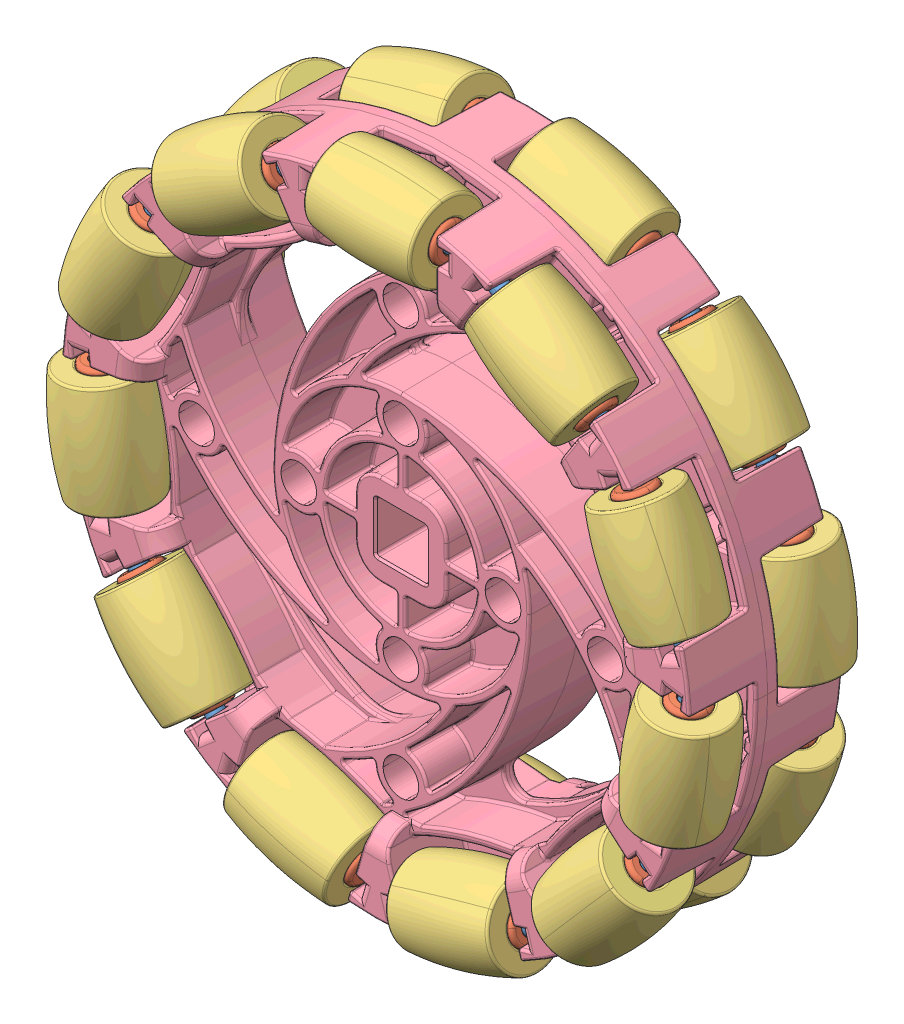
SolidWorks assembly 3.25_ Omni-Directional Wheel (276-3526) part, configuration Default. Lengths in mm.
Overall size (90.82 89.11 34).
90 component instances, 4 part files, 0 mates.
Components (placement in the parent):
- 3.25_ Omni-Directional Wheel (276-3526) .step-1: 3.25_ Omni-Directional Wheel (276-3526) .step [Default] at origin size (90.82 89.11 34)
  - Roller Assembly.step-1: Roller Assembly.step [Default] at (-0.0014 35.9575 7.1) x (0 0.963098 -0.269151) z (-1 0 0) size (14.05 14.05 18.75)
    - 276-3526-001 Rev 1.step-1: 276-3526-001 Rev 1.step [Default] at origin size (2 2 18.75)
    - 276-3526-003 Rev 1.step-1: 276-3526-003 Rev 1.step [Default] at origin size (6.15 6.15 14.2)
    - 276-3526-002 Rev 1.step-1: 276-3526-002 Rev 1.step [Default] x (0 0 1) z (-0.908956 0.416893 0) size (13.2 10.6 10.6)
  - Roller Assembly.step-2: Roller Assembly.step [Default] at (-19.4287 30.2567 7.1) x (0.421057 -0.655178 0.627258) z (-0.841254 -0.540641 0) size (14.05 14.05 18.75)
    - 276-3526-001 Rev 1.step-1: 276-3526-001 Rev 1.step [Default] at origin size (2 2 18.75)
    - 276-3526-003 Rev 1.step-1: 276-3526-003 Rev 1.step [Default] at origin size (6.15 6.15 14.2)
    - 276-3526-002 Rev 1.step-1: 276-3526-002 Rev 1.step [Default] x (0 0 1) z (-0.908956 0.416893 0) size (13.2 10.6 10.6)
  - Roller Assembly.step-3: Roller Assembly.step [Default] at (-35.5935 -5.1038 7.1) x (0.979746 0.140866 -0.142315) z (0.142315 -0.989821 0) size (14.05 14.05 18.75)
    - 276-3526-001 Rev 1.step-1: 276-3526-001 Rev 1.step [Default] at origin size (2 2 18.75)
    - 276-3526-003 Rev 1.step-1: 276-3526-003 Rev 1.step [Default] at origin size (6.15 6.15 14.2)
    - 276-3526-002 Rev 1.step-1: 276-3526-002 Rev 1.step [Default] x (0 0 1) z (-0.908956 0.416893 0) size (13.2 10.6 10.6)
  - Roller Assembly.step-4: Roller Assembly.step [Default] at (-10.1434 -34.4972 7.1) x (0.079373 0.27032 -0.959493) z (0.959493 -0.281733 0) size (14.05 14.05 18.75)
    - 276-3526-001 Rev 1.step-1: 276-3526-001 Rev 1.step [Default] at origin size (2 2 18.75)
    - 276-3526-003 Rev 1.step-1: 276-3526-003 Rev 1.step [Default] at origin size (6.15 6.15 14.2)
    - 276-3526-002 Rev 1.step-1: 276-3526-002 Rev 1.step [Default] x (0 0 1) z (-0.908956 0.416893 0) size (13.2 10.6 10.6)
  - Roller Assembly.step-5: Roller Assembly.step [Default] at (27.166 -23.5574 7.1) x (-0.355209 0.30779 -0.882662) z (0.654861 0.75575 0) size (14.05 14.05 18.75)
    - 276-3526-001 Rev 1.step-1: 276-3526-001 Rev 1.step [Default] at origin size (2 2 18.75)
    - 276-3526-003 Rev 1.step-1: 276-3526-003 Rev 1.step [Default] at origin size (6.15 6.15 14.2)
    - 276-3526-002 Rev 1.step-1: 276-3526-002 Rev 1.step [Default] x (0 0 1) z (-0.908956 0.416893 0) size (13.2 10.6 10.6)
  - Roller Assembly.step-6: Roller Assembly.step [Default] at (32.7138 14.9249 7.1) x (0.89908 0.410596 0.151875) z (-0.415415 0.909632 0) size (14.05 14.05 18.75)
    - 276-3526-001 Rev 1.step-1: 276-3526-001 Rev 1.step [Default] at origin size (2 2 18.75)
    - 276-3526-003 Rev 1.step-1: 276-3526-003 Rev 1.step [Default] at origin size (6.15 6.15 14.2)
    - 276-3526-002 Rev 1.step-1: 276-3526-002 Rev 1.step [Default] x (0 0 1) z (-0.908956 0.416893 0) size (13.2 10.6 10.6)
  - Roller Assembly.step-7: Roller Assembly.step [Default] at (19.4515 30.242 7.1) x (0.194707 0.302971 0.932898) z (-0.841254 0.540641 0) size (14.05 14.05 18.75)
    - 276-3526-001 Rev 1.step-1: 276-3526-001 Rev 1.step [Default] at origin size (2 2 18.75)
    - 276-3526-003 Rev 1.step-1: 276-3526-003 Rev 1.step [Default] at origin size (6.15 6.15 14.2)
    - 276-3526-002 Rev 1.step-1: 276-3526-002 Rev 1.step [Default] x (0 0 1) z (-0.908956 0.416893 0) size (13.2 10.6 10.6)
  - Roller Assembly.step-8: Roller Assembly.step [Default] at (-32.7025 14.9497 7.1) x (0.82743 -0.377875 0.415415) z (-0.415415 -0.909632 0) size (14.05 14.05 18.75)
    - 276-3526-001 Rev 1.step-1: 276-3526-001 Rev 1.step [Default] at origin size (2 2 18.75)
    - 276-3526-003 Rev 1.step-1: 276-3526-003 Rev 1.step [Default] at origin size (6.15 6.15 14.2)
    - 276-3526-002 Rev 1.step-1: 276-3526-002 Rev 1.step [Default] x (0 0 1) z (-0.908956 0.416893 0) size (13.2 10.6 10.6)
  - Roller Assembly.step-9: Roller Assembly.step [Default] at (-27.1838 -23.5369 7.1) x (0.578931 0.501646 -0.642799) z (0.654861 -0.75575 0) size (14.05 14.05 18.75)
    - 276-3526-001 Rev 1.step-1: 276-3526-001 Rev 1.step [Default] at origin size (2 2 18.75)
    - 276-3526-003 Rev 1.step-1: 276-3526-003 Rev 1.step [Default] at origin size (6.15 6.15 14.2)
    - 276-3526-002 Rev 1.step-1: 276-3526-002 Rev 1.step [Default] x (0 0 1) z (-0.908956 0.416893 0) size (13.2 10.6 10.6)
  - Roller Assembly.step-10: Roller Assembly.step [Default] at (10.1174 -34.5048 7.1) x (0.079373 -0.27032 -0.959493) z (0.959493 0.281733 0) size (14.05 14.05 18.75)
    - 276-3526-001 Rev 1.step-1: 276-3526-001 Rev 1.step [Default] at origin size (2 2 18.75)
    - 276-3526-003 Rev 1.step-1: 276-3526-003 Rev 1.step [Default] at origin size (6.15 6.15 14.2)
    - 276-3526-002 Rev 1.step-1: 276-3526-002 Rev 1.step [Default] x (0 0 1) z (-0.908956 0.416893 0) size (13.2 10.6 10.6)
  - Roller Assembly.step-11: Roller Assembly.step [Default] at (35.5896 -5.1307 7.1) x (0.988515 -0.142127 -0.05136) z (0.142315 0.989821 0) size (14.05 14.05 18.75)
    - 276-3526-001 Rev 1.step-1: 276-3526-001 Rev 1.step [Default] at origin size (2 2 18.75)
    - 276-3526-003 Rev 1.step-1: 276-3526-003 Rev 1.step [Default] at origin size (6.15 6.15 14.2)
    - 276-3526-002 Rev 1.step-1: 276-3526-002 Rev 1.step [Default] x (0 0 1) z (-0.908956 0.416893 0) size (13.2 10.6 10.6)
  - Roller Assembly.step-12: Roller Assembly.step [Default] at (10.1434 34.4972 -7.1) x (0.083119 0.283078 -0.955489) z (0.959493 -0.281733 0) size (14.05 14.05 18.75)
    - 276-3526-001 Rev 1.step-1: 276-3526-001 Rev 1.step [Default] at origin size (2 2 18.75)
    - 276-3526-003 Rev 1.step-1: 276-3526-003 Rev 1.step [Default] at origin size (6.15 6.15 14.2)
    - 276-3526-002 Rev 1.step-1: 276-3526-002 Rev 1.step [Default] x (0 0 1) z (-0.908956 0.416893 0) size (13.2 10.6 10.6)
  - Roller Assembly.step-13: Roller Assembly.step [Default] at (27.1838 23.5369 -7.1) x (0.582526 0.504762 -0.637086) z (0.654861 -0.75575 0) size (14.05 14.05 18.75)
    - 276-3526-001 Rev 1.step-1: 276-3526-001 Rev 1.step [Default] at origin size (2 2 18.75)
    - 276-3526-003 Rev 1.step-1: 276-3526-003 Rev 1.step [Default] at origin size (6.15 6.15 14.2)
    - 276-3526-002 Rev 1.step-1: 276-3526-002 Rev 1.step [Default] x (0 0 1) z (-0.908956 0.416893 0) size (13.2 10.6 10.6)
  - Roller Assembly.step-14: Roller Assembly.step [Default] at (35.5935 5.1038 -7.1) x (0.926341 0.133188 -0.352355) z (0.142315 -0.989821 0) size (14.05 14.05 18.75)
    - 276-3526-001 Rev 1.step-1: 276-3526-001 Rev 1.step [Default] at origin size (2 2 18.75)
    - 276-3526-003 Rev 1.step-1: 276-3526-003 Rev 1.step [Default] at origin size (6.15 6.15 14.2)
    - 276-3526-002 Rev 1.step-1: 276-3526-002 Rev 1.step [Default] x (0 0 1) z (-0.908956 0.416893 0) size (13.2 10.6 10.6)
  - Roller Assembly.step-15: Roller Assembly.step [Default] at (32.7025 -14.9497 -7.1) x (0.897398 -0.409828 0.163453) z (-0.415415 -0.909632 0) size (14.05 14.05 18.75)
    - 276-3526-001 Rev 1.step-1: 276-3526-001 Rev 1.step [Default] at origin size (2 2 18.75)
    - 276-3526-003 Rev 1.step-1: 276-3526-003 Rev 1.step [Default] at origin size (6.15 6.15 14.2)
    - 276-3526-002 Rev 1.step-1: 276-3526-002 Rev 1.step [Default] x (0 0 1) z (-0.908956 0.416893 0) size (13.2 10.6 10.6)
  - Roller Assembly.step-16: Roller Assembly.step [Default] at (19.4287 -30.2567 -7.1) x (0.277612 -0.431972 0.858098) z (-0.841254 -0.540641 0) size (14.05 14.05 18.75)
    - 276-3526-001 Rev 1.step-1: 276-3526-001 Rev 1.step [Default] at origin size (2 2 18.75)
    - 276-3526-003 Rev 1.step-1: 276-3526-003 Rev 1.step [Default] at origin size (6.15 6.15 14.2)
    - 276-3526-002 Rev 1.step-1: 276-3526-002 Rev 1.step [Default] x (0 0 1) z (-0.908956 0.416893 0) size (13.2 10.6 10.6)
  - Roller Assembly.step-17: Roller Assembly.step [Default] at (-0.0136 -35.9575 -7.1) x (0 -0.239919 0.970793) z (-1 0 0) size (14.05 14.05 18.75)
    - 276-3526-001 Rev 1.step-1: 276-3526-001 Rev 1.step [Default] at origin size (2 2 18.75)
    - 276-3526-003 Rev 1.step-1: 276-3526-003 Rev 1.step [Default] at origin size (6.15 6.15 14.2)
    - 276-3526-002 Rev 1.step-1: 276-3526-002 Rev 1.step [Default] x (0 0 1) z (-0.908956 0.416893 0) size (13.2 10.6 10.6)
  - Roller Assembly.step-18: Roller Assembly.step [Default] at (-19.4515 -30.242 -7.1) x (0.31008 0.482494 0.819176) z (-0.841254 0.540641 0) size (14.05 14.05 18.75)
    - 276-3526-001 Rev 1.step-1: 276-3526-001 Rev 1.step [Default] at origin size (2 2 18.75)
    - 276-3526-003 Rev 1.step-1: 276-3526-003 Rev 1.step [Default] at origin size (6.15 6.15 14.2)
    - 276-3526-002 Rev 1.step-1: 276-3526-002 Rev 1.step [Default] x (0 0 1) z (-0.908956 0.416893 0) size (13.2 10.6 10.6)
  - Roller Assembly.step-19: Roller Assembly.step [Default] at (-32.7138 -14.9249 -7.1) x (0.58758 0.268339 0.763377) z (-0.415415 0.909632 0) size (14.05 14.05 18.75)
    - 276-3526-001 Rev 1.step-1: 276-3526-001 Rev 1.step [Default] at origin size (2 2 18.75)
    - 276-3526-003 Rev 1.step-1: 276-3526-003 Rev 1.step [Default] at origin size (6.15 6.15 14.2)
    - 276-3526-002 Rev 1.step-1: 276-3526-002 Rev 1.step [Default] x (0 0 1) z (-0.908956 0.416893 0) size (13.2 10.6 10.6)
  - Roller Assembly.step-20: Roller Assembly.step [Default] at (-35.5896 5.1307 -7.1) x (0.965498 -0.138818 0.220323) z (0.142315 0.989821 0) size (14.05 14.05 18.75)
    - 276-3526-001 Rev 1.step-1: 276-3526-001 Rev 1.step [Default] at origin size (2 2 18.75)
    - 276-3526-003 Rev 1.step-1: 276-3526-003 Rev 1.step [Default] at origin size (6.15 6.15 14.2)
    - 276-3526-002 Rev 1.step-1: 276-3526-002 Rev 1.step [Default] x (0 0 1) z (-0.908956 0.416893 0) size (13.2 10.6 10.6)
  - Roller Assembly.step-21: Roller Assembly.step [Default] at (-27.166 23.5574 -7.1) x (0.75327 -0.652712 -0.080935) z (0.654861 0.75575 0) size (14.05 14.05 18.75)
    - 276-3526-001 Rev 1.step-1: 276-3526-001 Rev 1.step [Default] at origin size (2 2 18.75)
    - 276-3526-003 Rev 1.step-1: 276-3526-003 Rev 1.step [Default] at origin size (6.15 6.15 14.2)
    - 276-3526-002 Rev 1.step-1: 276-3526-002 Rev 1.step [Default] x (0 0 1) z (-0.908956 0.416893 0) size (13.2 10.6 10.6)
  - Roller Assembly.step-22: Roller Assembly.step [Default] at (-10.1174 34.5048 -7.1) x (0.123782 -0.421563 -0.898311) z (0.959493 0.281733 0) size (14.05 14.05 18.75)
    - 276-3526-001 Rev 1.step-1: 276-3526-001 Rev 1.step [Default] at origin size (2 2 18.75)
    - 276-3526-003 Rev 1.step-1: 276-3526-003 Rev 1.step [Default] at origin size (6.15 6.15 14.2)
    - 276-3526-002 Rev 1.step-1: 276-3526-002 Rev 1.step [Default] x (0 0 1) z (-0.908956 0.416893 0) size (13.2 10.6 10.6)
  - 276-3526-004 Rev 1.step-1: 276-3526-004 Rev 1.step [Default] at origin size (78.5 78.5 19.07)
